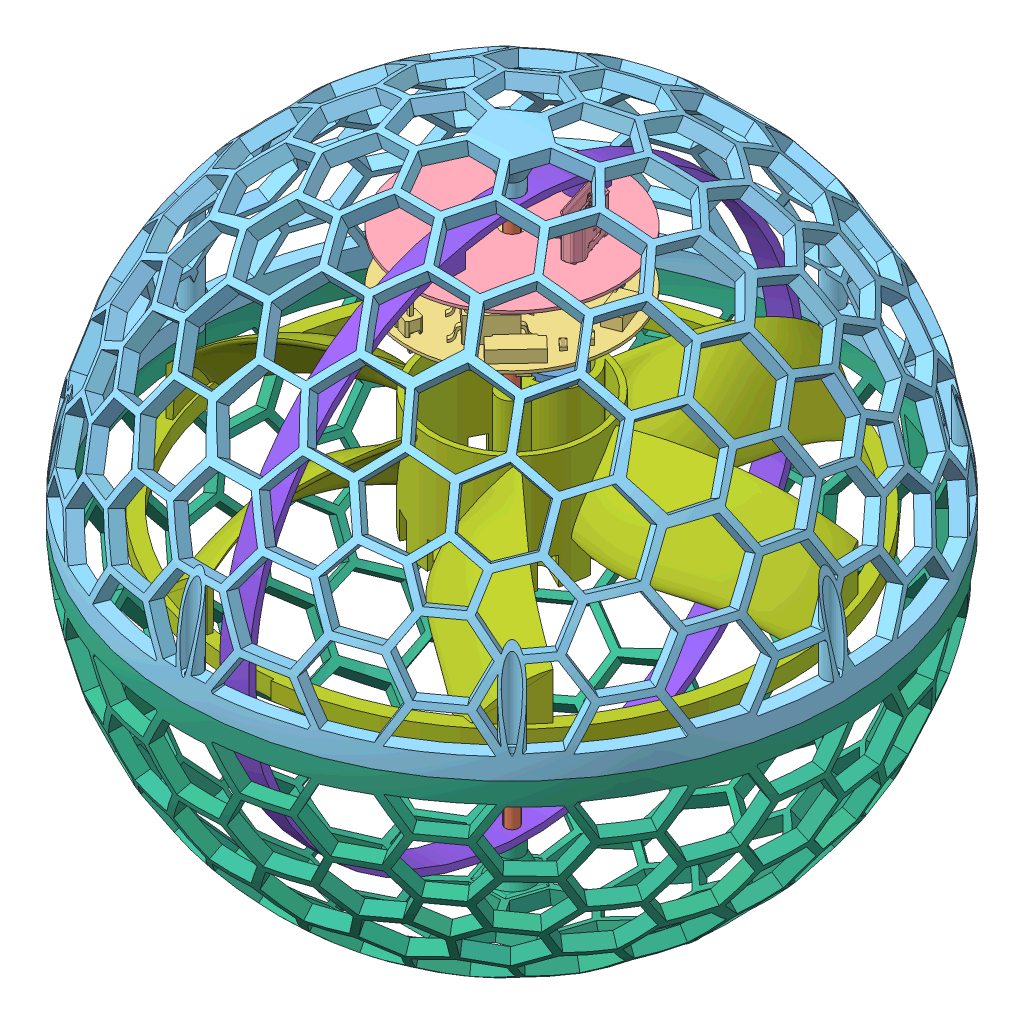
SolidWorks assembly HoverBall, configuration Default. Lengths in mm.
Overall size (95 95 95).
8 component instances, 8 part files, 15 mates.
Components (placement in the parent):
- motor-1: motor [Default] at (-48.9021 164.5346 210.6787) x (-0.837169 0 -0.546944) z (-0.546944 0 0.837169) size (7 21.6 7)
- Rod-1: Rod [Default] at (-48.5023 107.2383 217.4168) x (0.463763 0 -0.885959) z (0.885959 0 0.463763) size (1.9 87 1.9)
- HoverBall_main-1: HoverBall_main [Default] at (-48.5023 176.9249 217.4168) x (-0.686154 0 0.727456) z (0 1 0) size (30 30 8.7)
- HoverBall_power-1: HoverBall_power [Default] at (-48.5023 183.9982 217.4168) x (0.001724 0 -0.999999) z (0 -1 0) size (30 30 8.81)
- Polyhedron_holes-4: Polyhedron_holes [Default] at (-48.5023 148.6883 217.4168) size (95 47.5 95)
- Polyhedron_taps-2: Polyhedron_taps [Default] at (-48.5023 148.6883 217.4168) x (-1 0 0) z (0 0 1) size (95 47.5 95)
- motor hub - Copy-1: motor hub - Copy [Default] at (-48.5023 163.9346 217.4168) x (0.059224 0 0.998245) z (0.998245 0 -0.059224) size (79.62 18.5 78.75)
- LED ring-1: LED ring [Default] at (-48.5023 148.7083 217.4168) x (0.999999 0 0.001724) z (-0.001724 0 0.999999) size (82 90 90)
Mates (geometry in assembly coordinates):
- Concentric13: concentric aligned: cylinder of Rod-1 through (-48.5023 194.2383 217.4168) axis (0 -1 0) radius 0.95; circle of motor hub - Copy-1
- Coincident12: coincident anti-aligned: plane of motor-1 through (-49.0146 147.7346 210.6863) normal (0 -1 0); plane of motor hub - Copy-1 through (-48.5023 147.7346 217.4168) normal (0 1 0)
- Concentric14: concentric aligned: circle of motor-1; circle of motor hub - Copy-1
- Concentric16: concentric anti-aligned: circle of Rod-1; circle of LED ring-1
- Coincident13: coincident anti-aligned: plane of Polyhedron_holes-4 through (-48.5023 148.6883 217.4168) normal (0 -1 0); plane of Polyhedron_taps-2 through (-48.5023 148.6883 217.4168) normal (0 1 0)
- Concentric17: concentric anti-aligned: circle of Polyhedron_holes-4; circle of Polyhedron_taps-2
- Concentric18: concentric anti-aligned: circle of Polyhedron_holes-4; circle of Polyhedron_taps-2
- Concentric19: concentric aligned: circle of Rod-1; circle of Polyhedron_holes-4
- Coincident15: coincident anti-aligned: plane of Rod-1 through (-48.5023 194.2383 217.4168) normal (0 1 0); plane of Polyhedron_holes-4 through (-48.5023 194.2383 217.4168) normal (0 -1 0)
- Distance1: distance = 25.0036 mm anti-aligned: plane of motor hub - Copy-1 through (-48.5023 163.9346 217.4168) normal (0 1 0); plane of Polyhedron_holes-4 through (-48.5023 188.9383 217.4168) normal (0 -1 0)
- Concentric20: concentric aligned: cylinder of Rod-1 through (-48.5023 194.2383 217.4168) axis (0 -1 0) radius 0.95; circle of HoverBall_power-1
- Concentric21: concentric anti-aligned: cylinder of Rod-1 through (-48.5023 194.2383 217.4168) axis (0 -1 0) radius 0.95; circle of HoverBall_main-1
- Coincident17: coincident anti-aligned: plane of HoverBall_power-1 through (-60.6313 184.4083 226.2423) normal (0 1 0); plane of LED ring-1 through (-56.9926 184.4083 223.5947) normal (0 -1 0)
- Concentric23: concentric aligned: circle of HoverBall_power-1; circle of LED ring-1
- Distance2: distance = 0.23 mm anti-aligned: sphere of LED ring-1; plane of Polyhedron_holes-4 through (-48.5023 188.9383 217.4168) normal (0 -1 0)
